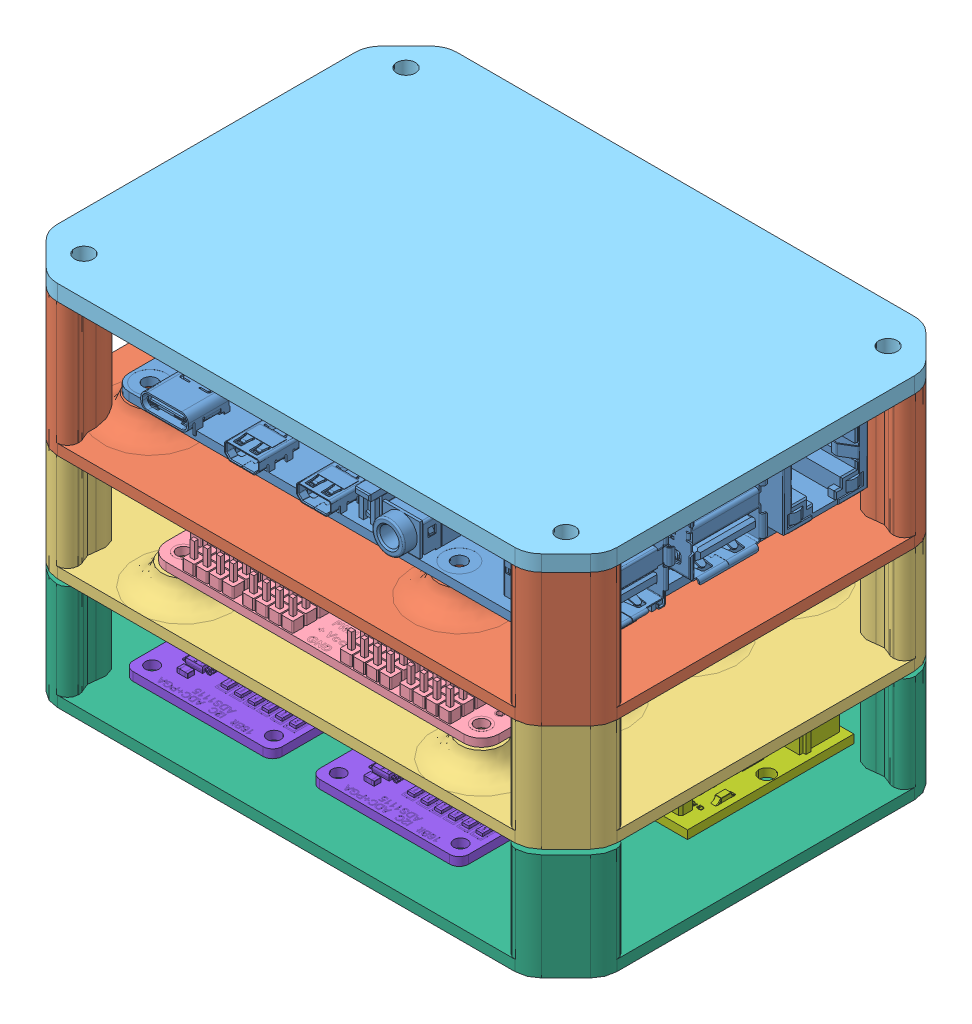
SolidWorks assembly ASM-BOX, configuration По умолчанию. Lengths in mm.
Overall size (105 68.92 75).
15 component instances, 8 part files, 20 mates.
Components (placement in the parent):
- Raspberry Pi 4 Model B-1: Raspberry Pi 4 Model B [По умолчанию] at origin size (88.99 19.91 58.4)
- level-0-1: level-0 [По умолчанию] at (-0.5 -6.79 0) x (1 0 0) z (0 1 0) size (105 75 25)
- level-1-1: level-1 [По умолчанию] at (-0.5 -26.79 0) x (-1 0 0) z (0 1 0) size (105 75 20)
- 12Channel PWM-1: 12Channel PWM [Default] at (-0.5 -20.79 19.4) x (0 0 -1) z (1 0 0) size (25.4 7.55 66.7)
- 12Channel PWM-2: 12Channel PWM [Default] at (-0.5 -20.79 -19.4) x (0 0 1) z (-1 0 0) size (25.4 7.55 66.7)
- cap-1: cap [По умолчанию] at (-0.5 18.21 0) x (1 0 0) z (0 1 0) size (105 75 3)
- level-2-1: level-2 [По умолчанию] at (-0.5 -47.7068 0) x (-1 0 0) z (0 1 0) size (105 75 20)
- ACS712.step-1: ACS712.step [По умолчанию] at (36.5252 -41.7068 -9.7273) x (0 0 -1) z (1 0 0) size (31.19 12.78 13.3)
- ACS712.step-2: ACS712.step [По умолчанию] at (21.5252 -41.7068 -9.7273) x (0 0 -1) z (1 0 0) size (31.19 12.78 13.3)
- ACS712.step-3: ACS712.step [По умолчанию] at (6.5252 -41.7068 -9.7273) x (0 0 -1) z (1 0 0) size (31.19 12.78 13.3)
- ACS712.step-4: ACS712.step [По умолчанию] at (-8.4748 -41.7068 -9.7273) x (0 0 -1) z (1 0 0) size (31.19 12.78 13.3)
- ACS712.step-5: ACS712.step [По умолчанию] at (-23.4748 -41.7068 -9.7273) x (0 0 -1) z (1 0 0) size (31.19 12.78 13.3)
- ACS712.step-6: ACS712.step [По умолчанию] at (-38.4748 -41.7068 -9.7273) x (0 0 -1) z (1 0 0) size (31.19 12.78 13.3)
- 16Bit I2C ADC+PGA - ADS1115-1: 16Bit I2C ADC+PGA - ADS1115 [По умолчанию] at (-22.3293 -41.7068 23.5308) x (-1 0 0) z (0 1 0) size (27.94 17.27 2.74)
- 16Bit I2C ADC+PGA - ADS1115-2: 16Bit I2C ADC+PGA - ADS1115 [По умолчанию] at (12.6707 -41.7068 23.5308) x (-1 0 0) z (0 1 0) size (27.94 17.27 2.74)
Mates (geometry in assembly coordinates):
- Концентричный1: concentric aligned: cylinder of Raspberry Pi 4 Model B-1 through (-39 0.8 24.5) axis (0 1 0) radius 1.35; cylinder of level-0-1 through (-39 -6.79 24.5) axis (0 1 0) radius 2.5
- Концентричный2: concentric aligned: cylinder of Raspberry Pi 4 Model B-1 through (-39 0.8 -24.5) axis (0 1 0) radius 1.35; cylinder of level-0-1 through (-39 -6.79 -24.5) axis (0 1 0) radius 2.5
- Совпадение1: coincident anti-aligned: plane of Raspberry Pi 4 Model B-1 through (-39 -0.79 -24.5) normal (0 -1 0); plane of level-0-1 through (-39 -0.79 -24.5) normal (0 1 0)
- Концентричный3: concentric aligned: cylinder of level-0-1 through (-45.7145 -15.79 30.2145) axis (0 1 0) radius 1.75; cylinder of level-1-1 through (-45.7145 -40.79 30.2145) axis (0 1 0) radius 1.75
- Совпадение2: coincident aligned: plane of level-0-1 through (-53 18.21 -30) normal (-0.707107 0 -0.707107); plane of level-1-1 through (-45.5 -6.79 -37.5) normal (-0.707107 0 -0.707107)
- Совпадение3: coincident anti-aligned: plane of level-0-1 through (-0.5 -6.79 0) normal (0 -1 0); plane of level-1-1 through (-0.5 -6.79 0) normal (0 1 0)
- Концентричный4: concentric aligned: cylinder of level-1-1 through (-28.45 -26.79 10) axis (0 1 0) radius 2.5; cylinder of 12Channel PWM-1 through (-28.45 -24.3255 10) axis (0 1 0) radius 1.25
- Концентричный5: concentric aligned: cylinder of level-1-1 through (-28.45 -26.79 28.8) axis (0 1 0) radius 2.5; cylinder of 12Channel PWM-1 through (-28.45 -24.3255 28.8) axis (0 1 0) radius 1.25
- Совпадение4: coincident anti-aligned: plane of level-1-1 through (-28.45 -20.79 28.8) normal (0 1 0); plane of 12Channel PWM-1 through (-28.45 -20.79 10) normal (0 -1 0)
- Концентричный6: concentric aligned: cylinder of level-1-1 through (-28.45 -26.79 -28.8) axis (0 1 0) radius 2.5; cylinder of 12Channel PWM-2 through (-28.45 -24.3255 -28.8) axis (0 1 0) radius 1.25
- Концентричный7: concentric aligned: cylinder of level-1-1 through (-28.45 -26.79 -10) axis (0 1 0) radius 2.5; cylinder of 12Channel PWM-2 through (-28.45 -24.3255 -10) axis (0 1 0) radius 1.25
- Совпадение5: coincident anti-aligned: plane of level-1-1 through (-28.45 -20.79 -28.8) normal (0 1 0); plane of 12Channel PWM-2 through (27.45 -20.79 -10) normal (0 -1 0)
- Концентричный8: concentric anti-aligned: cylinder of level-0-1 through (-45.7145 -15.79 -30.2145) axis (0 1 0) radius 1.75; cylinder of cap-1 through (-45.7145 21.21 -30.2145) axis (0 -1 0) radius 1.75
- Концентричный9: concentric anti-aligned: cylinder of level-0-1 through (44.7145 -15.79 -30.2145) axis (0 1 0) radius 1.75; cylinder of cap-1 through (44.7145 21.21 -30.2145) axis (0 -1 0) radius 1.75
- Совпадение6: coincident anti-aligned: plane of level-0-1 through (-0.5 18.21 0) normal (0 1 0); plane of cap-1 through (-43.4289 18.21 32.5) normal (0 -1 0)
- Совпадение7: coincident anti-aligned: plane of level-0-1 through (-0.5 -6.79 0) normal (0 -1 0); plane of level-1-1 through (-0.5 -6.79 0) normal (0 1 0)
- Концентричный10: concentric aligned: cylinder of level-1-1 through (44.7145 -40.79 30.2145) axis (0 1 0) radius 1.75; cylinder of level-2-1 through (44.7145 -61.7068 30.2145) axis (0 1 0) radius 1.75
- Концентричный11: concentric aligned: cylinder of level-1-1 through (44.7145 -40.79 -30.2145) axis (0 1 0) radius 1.75; cylinder of level-2-1 through (44.7145 -61.7068 -30.2145) axis (0 1 0) radius 1.75
- Расстояние1: distance = 4 mm anti-aligned: plane of 16Bit I2C ADC+PGA - ADS1115-1 through (-22.3293 -41.7068 23.5308) normal (0 -1 0); plane of level-2-1 through (-0.5 -45.7068 0) normal (0 1 0)
- Расстояние2: distance = 4 mm anti-aligned: plane of ACS712.step-6 through (-38.4748 -41.7068 -9.7273) normal (0 -1 0); plane of level-2-1 through (-0.5 -45.7068 0) normal (0 1 0)
